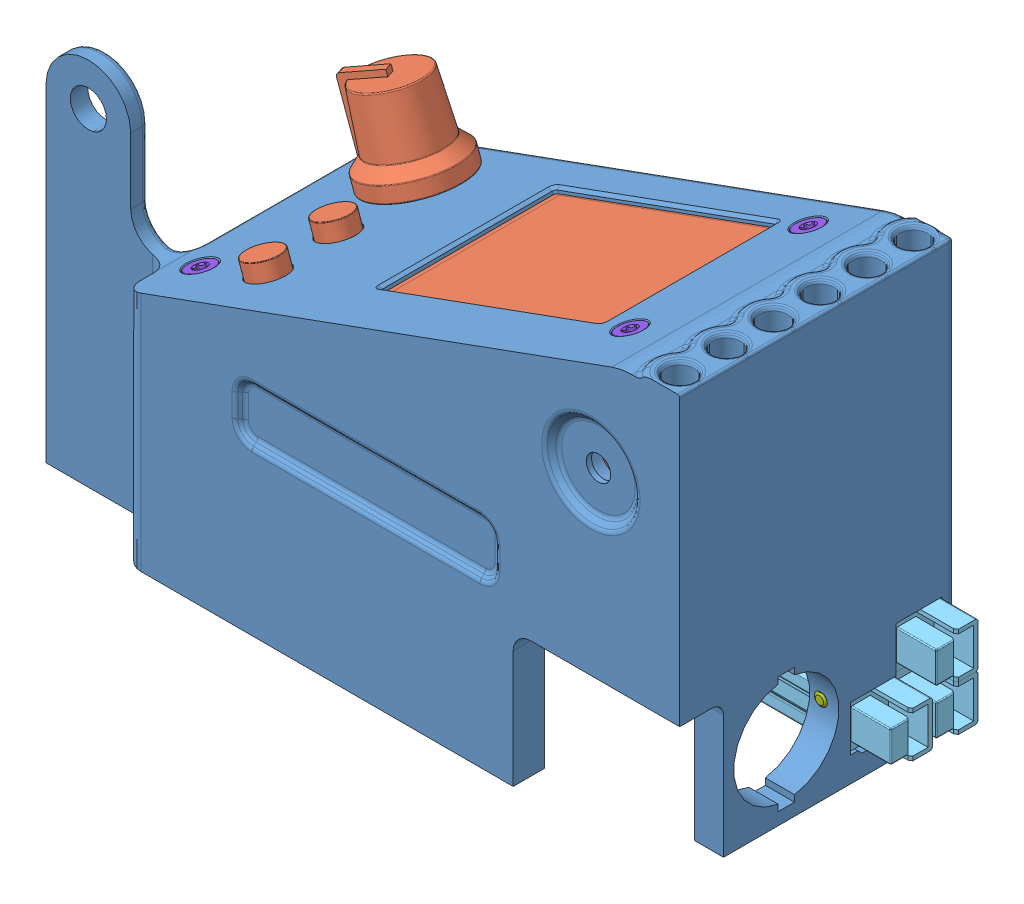
SolidWorks assembly AxxSolder_JBC-ADS, configuration Default. Lengths in mm.
Overall size (122.65 83.92 49.52).
14 component instances, 8 part files, 21 mates.
Components (placement in the parent):
- Encolsure_JBC-ADS-1: Encolsure_JBC-ADS [Default] x (-1 0 0) z (0 0 -1) size (116.45 72.32 47.1)
- AxxSolder-1: AxxSolder [Default] at (-85.4212 30.7371 -5.6) x (0 0 1) z (-0.34202 0.939693 0) size (39.06 82.54 35.41)
- Mounting_Bracket_A-1: Mounting_Bracket_A [Default] at (-81.2341 28.0043 -25.1) x (0 0 1) z (0.939693 0.34202 0) size (37.5 7 4.5)
- Mounting_Bracket_B-1: Mounting_Bracket_B [Default] at (-8.8758 54.3406 -25.08) x (0 0 1) z (0.939693 0.34202 0) size (34.98 7 4.5)
- Anderson_PowerPole-1: Anderson_PowerPole [Default] at (-12.4461 6.6141 -40.9285) x (0 -1 0) z (1 0 0) size (16.24 16.24 22.71)
  - powerpole 15-45A housing.step-3: powerpole 15-45A housing.step [Default] at origin size (8.44 8.44 22.71)
  - powerpole 15-45A housing.step-5: powerpole 15-45A housing.step [Default] at (-7.8 0 0) size (8.44 8.44 22.71)
  - powerpole 15-45A housing.step-6: powerpole 15-45A housing.step [Default] at (0 -7.8 0) size (8.44 8.44 22.71)
- Mini Rocker 4-Pin Switch-1: Mini Rocker 4-Pin Switch [Default] at (-90.2 12.3 -37.7) x (0 0 -1) z (0 1 0) size (15.2 28.43 21.2)
- 91292A019_18-8 Stainless Steel Socket Head Screw-1: 91292A019_18-8 Stainless Steel Socket Head Screw [91292A019] at (2 10.5 -26.9) size (4.5 4.5 22.72)
- 92703A451_18-8 Stainless Steel Torx Flat Head Screws-1: 92703A451_18-8 Stainless Steel Torx Flat Head Screws [92703A451] at (-13.3385 66.4495 -9.86) x (0.883022 0.321394 0.34202) z (-0.34202 0.939693 0) size (4.7 4.7 12.12)
- 92703A451_18-8 Stainless Steel Torx Flat Head Screws-2: 92703A451_18-8 Stainless Steel Torx Flat Head Screws [92703A451] at (-13.3385 66.4495 -40.34) x (0.883022 0.321394 0.34202) z (-0.34202 0.939693 0) size (4.7 4.7 12.12)
- 92703A451_18-8 Stainless Steel Torx Flat Head Screws-3: 92703A451_18-8 Stainless Steel Torx Flat Head Screws [92703A451] at (-85.6478 40.1311 -41.6) x (0.883022 0.321394 0.34202) z (-0.34202 0.939693 0) size (4.7 4.7 12.12)
- 92703A451_18-8 Stainless Steel Torx Flat Head Screws-4: 92703A451_18-8 Stainless Steel Torx Flat Head Screws [92703A451] at (-85.6478 40.1311 -8.6) x (0.883022 0.321394 0.34202) z (-0.34202 0.939693 0) size (4.7 4.7 12.12)
Mates (geometry in assembly coordinates):
- Coincident1: coincident anti-aligned: plane of Encolsure_JBC-ADS-1 through (0 0 -44.85) normal (0 0 1); plane of Anderson_PowerPole-1/powerpole 15-45A housing.step-5 through (11.2 18.3 -44.85) normal (0 0 -1)
- Coincident3: coincident anti-aligned: plane of Encolsure_JBC-AD-SF-1 through (2 2.7 -44.85) normal (0 1 0); plane of Anderson_PowerPole-1/powerpole 15-45A housing.step-6 through (11.2 2.7 -37.05) normal (0 -1 0)
- Distance2: distance = 6.2 mm aligned: plane of Anderson_PowerPole-1/powerpole 15-45A housing.step-3 through (11.2 10.5 -37.05) normal (1 0 0); plane of Encolsure_JBC-ADS-1 through (5 0 -91.3832) normal (1 0 0)
- Concentric1: concentric aligned: cylinder of Encolsure_JBC-ADS-1 through (-82.2601 30.8234 -41.6) axis (-0.34202 0.939693 0) radius 1.25; cylinder of AxxSolder-1 through (-82.5987 31.7537 -41.6) axis (-0.34202 0.939693 0) radius 1.25
- Coincident4: coincident anti-aligned: plane of Encolsure_JBC-ADS-1 through (-80.2833 34.3098 -43.85) normal (0.34202 -0.939693 0); plane of AxxSolder-1 through (-47.2061 46.3489 -25.1) normal (-0.34202 0.939693 0)
- Coincident5: coincident anti-aligned: plane of AxxSolder-1 through (-46.6589 44.8454 -25.1) normal (0.34202 -0.939693 0); plane of Mounting_Bracket_A-1 through (-82.6021 31.7631 -25.1) normal (-0.34202 0.939693 0)
- Concentric3: concentric aligned: cylinder of AxxSolder-1 through (-82.5987 31.7537 -41.6) axis (-0.34202 0.939693 0) radius 1.25; cylinder of Mounting_Bracket_A-1 through (-80.208 25.1853 -41.6) axis (-0.34202 0.939693 0) radius 1
- Concentric4: concentric aligned: cylinder of AxxSolder-1 through (-10.2405 58.09 -40.32) axis (-0.34202 0.939693 0) radius 1.25; cylinder of Mounting_Bracket_B-1 through (-7.8498 51.5215 -40.32) axis (-0.34202 0.939693 0) radius 1
- Coincident6: coincident anti-aligned: plane of AxxSolder-1 through (-46.6589 44.8454 -25.1) normal (0.34202 -0.939693 0); plane of Mounting_Bracket_B-1 through (-10.2439 58.0994 -25.08) normal (-0.34202 0.939693 0)
- Coincident7: coincident anti-aligned: plane of Encolsure_JBC-ADS-1 through (-90.2 69.6 -11) normal (-1 0 0); plane of Mini Rocker 4-Pin Switch-1 through (-90.2 12.3 -37.7) normal (1 0 0)
- Width1: width anti-aligned: plane of Encolsure_JBC-ADS-1 through (-91.2034 22.2 -31.3) normal (0 0 -1); plane of Encolsure_JBC-ADS-1 through (-91.2034 22.2 -44.1) normal (0 0 1); plane of Mini Rocker 4-Pin Switch-1 through (-92.3 1.7 -30.1) normal (0 0 1); plane of Mini Rocker 4-Pin Switch-1 through (-92.3 1.7 -45.3) normal (0 0 -1)
- Width2: width anti-aligned: plane of Mini Rocker 4-Pin Switch-1 through (-92.3 1.7 -30.1) normal (0 -1 0); plane of Mini Rocker 4-Pin Switch-1 through (-92.3 22.9 -30.1) normal (0 1 0); plane of Encolsure_JBC-ADS-1 through (-91.2034 2.4 -44.1) normal (0 1 0); plane of Encolsure_JBC-ADS-1 through (-91.2034 22.2 -44.1) normal (0 -1 0)
- Coincident8: coincident anti-aligned: plane of Encolsure_JBC-ADS-1 through (0 0 0) normal (0 0 -1)
- Coincident9: coincident aligned: plane of Encolsure_JBC-ADS-1 through (0 0 0) normal (0 1 0)
- Coincident10: coincident anti-aligned: plane of Encolsure_JBC-ADS-1 through (0 0 0) normal (-1 0 0)
- Coincident11: coincident aligned: cone of Encolsure_JBC-ADS-1 through (-85.6803 40.2203 -8.6) axis (0.34202 -0.939693 0); cone of 92703A451_18-8 Stainless Steel Torx Flat Head Screws-4 through (-85.1348 38.7215 -8.6) axis (0.34202 -0.939693 0)
- Coincident12: coincident aligned: cone of Encolsure_JBC-ADS-1 through (-85.6803 40.2203 -41.6) axis (0.34202 -0.939693 0); cone of 92703A451_18-8 Stainless Steel Torx Flat Head Screws-3 through (-85.1348 38.7215 -41.6) axis (0.34202 -0.939693 0)
- Coincident13: coincident aligned: cone of Encolsure_JBC-ADS-1 through (-13.371 66.5388 -40.34) axis (0.34202 -0.939693 0); cone of 92703A451_18-8 Stainless Steel Torx Flat Head Screws-2 through (-12.8254 65.04 -40.34) axis (0.34202 -0.939693 0)
- Coincident14: coincident aligned: cone of Encolsure_JBC-ADS-1 through (-13.371 66.5388 -9.86) axis (0.34202 -0.939693 0); cone of 92703A451_18-8 Stainless Steel Torx Flat Head Screws-1 through (-12.8254 65.04 -9.86) axis (0.34202 -0.939693 0)
- Concentric5: concentric anti-aligned: cylinder of Encolsure_JBC-ADS-1 through (2 10.5 -42.1) axis (0 0 -1) radius 1.25; cylinder of 91292A019_18-8 Stainless Steel Socket Head Screw-1 through (2 10.5 -49.4) axis (0 0 1) radius 2.25
- Coincident15: coincident anti-aligned: plane of Encolsure_JBC-ADS-1 through (2 10.5 -46.9) normal (0 0 -1); plane of 91292A019_18-8 Stainless Steel Socket Head Screw-1 through (2 10.5 -46.9) normal (0 0 1)
